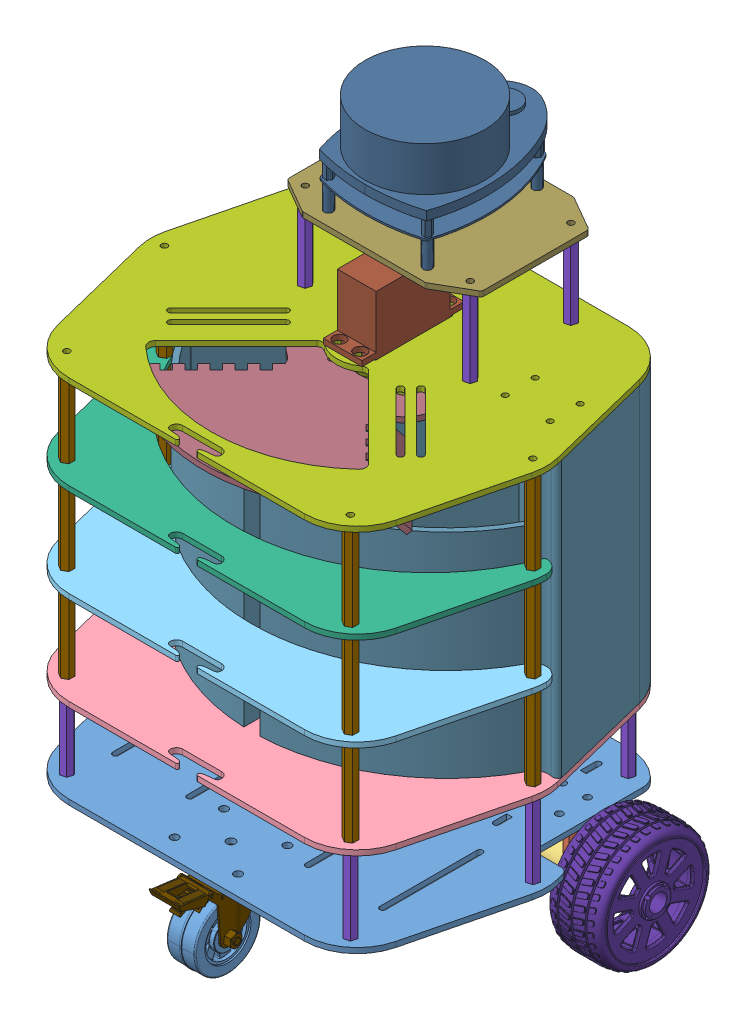
SolidWorks assembly 装配体1, configuration 默认. Lengths in mm.
Overall size (255.2 380.4 208.91).
45 component instances, 21 part files, 94 mates.
Components (placement in the parent):
- 底板1-1: 底板1 [默认] at origin size (224.29 3 183.94)
- 电机支架-1: 电机支架 [默认] at (90.25 -20.75 -110.5986) x (-1 0 0) z (0 0 1) size (33 34 26.5)
- 电机-1: 电机 [默认] at (36.95 -20.75 -110.5986) size (71 25.53 25.53)
- 电机-2: 电机 [默认] at (-36.95 -20.75 -110.5986) x (-1 0 0) z (0 0 -1) size (71 25.53 25.53)
- 电机支架-2: 电机支架 [默认] at (-90.25 -20.75 -110.5986) x (1 0 0) z (0 0 -1) size (33 34 26.5)
- 底板2-1: 底板2 [默认] at (0 48 0) size (224.29 3 183.94)
- 底板3-1: 底板3 [默认] at (0 101 0) size (224.29 3 99.61)
- 底板4-1: 底板4 [默认] at (0 154 0) size (224.29 3 99.54)
- 底板5-1: 底板5 [默认] at (0 207 0) size (224.29 3 183.94)
- 铜柱45-1: 铜柱45 [默认] at (80.4502 3 16.819) size (6.73 45 6.65)
- 铜柱45-2: 铜柱45 [默认] at (104.5075 3 -62.6242) size (6.73 45 6.65)
- 铜柱45-4: 铜柱45 [默认] at (-80.4502 3 16.819) size (6.73 45 6.65)
- 铜柱45-5: 铜柱45 [默认] at (-104.5075 3 -62.6242) size (6.73 45 6.65)
- 铜柱45-6: 铜柱45 [默认] at (-79.5 3 -141.7823) size (6.73 45 6.65)
- 铜柱45-7: 铜柱45 [默认] at (79.5 3 -141.7823) size (6.73 45 6.65)
- 铜柱50-1: 铜柱50 [默认] at (104.5075 157 -62.6242) size (6.07 50 6.93)
- 铜柱50-2: 铜柱50 [默认] at (-80.4502 51 16.819) size (6.07 50 6.93)
- 铜柱50-3: 铜柱50 [默认] at (-104.5075 51 -62.6242) size (6.07 50 6.93)
- 铜柱50-4: 铜柱50 [默认] at (80.4502 51 16.819) size (6.07 50 6.93)
- 铜柱50-5: 铜柱50 [默认] at (-104.5075 104 -62.6242) size (6.07 50 6.93)
- 铜柱50-6: 铜柱50 [默认] at (-80.4502 104 16.819) size (6.07 50 6.93)
- 铜柱50-7: 铜柱50 [默认] at (104.5075 51 -62.6242) size (6.07 50 6.93)
- 铜柱50-8: 铜柱50 [默认] at (80.4502 104 16.819) size (6.07 50 6.93)
- 铜柱50-9: 铜柱50 [默认] at (-80.4502 157 16.819) size (6.07 50 6.93)
- 铜柱50-10: 铜柱50 [默认] at (104.5075 104 -62.6242) size (6.07 50 6.93)
- 铜柱50-11: 铜柱50 [默认] at (-104.5075 157 -62.6242) size (6.07 50 6.93)
- 铜柱50-12: 铜柱50 [默认] at (80.4502 157 16.819) size (6.07 50 6.93)
- 激光雷达X4-1: 激光雷达X4 [默认] at (0 258 -120.1085) x (-1 0 0) z (0 0 -1) size (70.42 57 94.61)
- 舵机-1: 舵机 [默认] at (0 243 -88.1867) x (0 0 -1) z (-1 0 0) size (58 50 22)
- 底板6-1: 底板6 [默认] at (0.7291 255 -93.893) x (1 0 0) z (0 1 0) size (110.33 83.99 3)
- 铜柱45-8: 铜柱45 [默认] at (47.5277 210 -141.1486) size (6.73 45 6.65)
- 铜柱45-9: 铜柱45 [默认] at (-46.0695 210 -84.051) size (6.73 45 6.65)
- 铜柱45-10: 铜柱45 [默认] at (-46.0695 210 -141.1486) size (6.73 45 6.65)
- 铜柱45-11: 铜柱45 [默认] at (47.5277 210 -84.051) size (6.73 45 6.65)
- 乘物-1: 乘物 [默认] at (-0.1354 193 -20.9339) size (143.43 24.32 112.61)
- 垃圾桶-1: 垃圾桶 [默认] at (0.1354 51 -61.3346) size (220.93 156 146.93)
- 铜柱156-1: 铜柱156 [默认] at (0 51 -131.5682) size (6.91 156 6.21)
- 铜柱156-2: 铜柱156 [默认] at (0 51 -144.0797) size (6.91 156 6.21)
- 一字摇臂-1: 一字摇臂 [默认] at (0 193 -73.9628) x (1 0 0) z (0 1 0) size (47 9.8 7.5)
- 乘物2-1: 乘物2 [默认] at (47.7312 192.1451 -37.8905) x (0.651005 -0.382877 -0.655438) z (0.685403 -0.074582 0.724335) size (19.13 3 48.09) (hidden)
- 轮子酷-1: 轮子酷 [Default] at (-135.2789 -20.75 -110.5986) x (0 0.249093 0.96848) z (-1 0 0) size (66.95 66.95 31.63)
- 轮子酷-2: 轮子酷 [Default] at (135.2789 -20.75 -110.5986) x (0 0.432005 -0.901871) z (1 0 0) size (66.95 66.95 31.63)
- 万向-1: 万向 [默认] at (0 0 4.1514) x (0 0 -1) z (1 0 0) size (55.67 39.63 29.93)
- 万向新轮子-1: 万向新轮子 [默认] at (0.0227 -0.0918 24.1728) x (0 -0.009175 0.999958) z (-1 0 0) size (46.01 53.63 29.93)
- IMU-1: IMU [默认] at (-36.2463 19.5 -94.4147) size (55 18.5 65)
Mates (geometry in assembly coordinates):
- 同心1: concentric anti-aligned: cylinder of 电机支架-1 through (86.95 -20.75 -110.5986) axis (1 0 0) radius 4; cylinder of 电机-1 through (98.95 -20.75 -110.5986) axis (-1 0 0) radius 2
- 同心2: concentric aligned: cylinder of 电机支架-1 through (86.95 -20.75 -119.0986) axis (1 0 0) radius 1.5; cylinder of 电机-1 through (83.95 -20.75 -119.0986) axis (1 0 0) radius 1.5
- 重合1: coincident anti-aligned: plane of 电机支架-1 through (86.95 -20.75 -110.5986) normal (-1 0 0); plane of 电机-1 through (86.95 -20.75 -110.5986) normal (1 0 0)
- 重合3: coincident anti-aligned: plane of 底板1-1 through (0 0 0) normal (0 -1 0); plane of 电机支架-1 through (86.95 0 -97.3486) normal (0 1 0)
- 重合5: coincident anti-aligned: plane of 电机-2 through (-86.95 -20.75 -110.5986) normal (-1 0 0); plane of 电机支架-2 through (-86.95 -20.75 -110.5986) normal (1 0 0)
- 同心4: concentric anti-aligned: cylinder of 电机-2 through (-98.95 -20.75 -110.5986) axis (1 0 0) radius 2; cylinder of 电机支架-2 through (-86.95 -20.75 -110.5986) axis (-1 0 0) radius 4
- 同心6: concentric aligned: cylinder of 电机-2 through (-83.95 -20.75 -102.0986) axis (-1 0 0) radius 1.5; cylinder of 电机支架-2 through (-86.95 -20.75 -102.0986) axis (-1 0 0) radius 1.5
- 重合6: coincident aligned: plane of 底板1-1 through (90.25 3 0) normal (1 0 0); plane of 电机支架-1 through (90.25 -20.75 -110.5986) normal (1 0 0)
- 重合7: coincident anti-aligned: plane of 底板1-1 through (0 0 0) normal (0 -1 0); plane of 电机支架-2 through (-86.95 0 -123.8486) normal (0 1 0)
- 重合8: coincident aligned: plane of 底板1-1 through (-90.25 3 0) normal (-1 0 0); plane of 电机支架-2 through (-90.25 -20.75 -110.5986) normal (-1 0 0)
- 重合9: coincident aligned: plane of 电机支架-1 through (86.95 0 -123.8486) normal (0 0 -1); plane of 电机支架-2 through (-86.95 -20.75 -123.8486) normal (0 0 -1)
- 距离4: distance = 30.7453 mm aligned: plane of 电机支架-1 through (86.95 0 -123.8486) normal (0 0 -1); plane of 底板1-1 through (0 3 -154.594) normal (0 0 -1)
- 重合15: coincident aligned: plane of 底板1-1 through (91.8773 3 22.7831) normal (0.970604 0 0.240684); plane of 底板2-1 through (91.8773 51 22.7831) normal (0.970604 0 0.240684)
- 重合16: coincident aligned: plane of 底板1-1 through (0 3 29.3457) normal (0 0 1); plane of 底板2-1 through (0 51 29.3457) normal (0 0 1)
- 距离6: distance = 45 mm anti-aligned: plane of 底板1-1 through (0 3 0) normal (0 1 0); plane of 底板2-1 through (0 48 0) normal (0 -1 0)
- 重合18: coincident aligned: plane of 底板2-1 through (0 51 29.3457) normal (0 0 1); plane of 底板3-1 through (0 104 29.3457) normal (0 0 1)
- 重合19: coincident aligned: plane of 底板2-1 through (91.8773 51 22.7831) normal (0.970604 0 0.240684); plane of 底板3-1 through (91.8773 104 22.7831) normal (0.970604 0 0.240684)
- 重合20: coincident aligned: plane of 底板3-1 through (0 104 29.3457) normal (0 0 1); plane of 底板4-1 through (0 157 29.3457) normal (0 0 1)
- 重合21: coincident: plane of 底板3-1 through (91.8773 104 22.7831) normal (0.970604 0 0.240684); line of 底板4-1 through (95.8987 157 6.5662) axis (0.240684 0 -0.970604)
- 重合22: coincident aligned: plane of 底板4-1 through (91.8773 157 22.7831) normal (0.970604 0 0.240684); plane of 底板5-1 through (91.8773 210 22.7831) normal (0.970604 0 0.240684)
- 重合23: coincident aligned: plane of 底板4-1 through (0 157 29.3457) normal (0 0 1); plane of 底板5-1 through (0 210 29.3457) normal (0 0 1)
- 距离7: distance = 50 mm anti-aligned: plane of 底板2-1 through (0 51 0) normal (0 1 0); plane of 底板3-1 through (0 101 0) normal (0 -1 0)
- 距离8: distance = 50 mm anti-aligned: plane of 底板3-1 through (0 104 0) normal (0 1 0); plane of 底板4-1 through (0 154 0) normal (0 -1 0)
- 距离9: distance = 50 mm anti-aligned: plane of 底板5-1 through (0 207 0) normal (0 -1 0); plane of 底板4-1 through (0 157 0) normal (0 1 0)
- 同心8: concentric anti-aligned: cylinder of 底板2-1 through (104.5075 41 -62.6242) axis (0 1 0) radius 1.75; cylinder of 铜柱45-2 through (104.5075 48 -62.6242) axis (0 -1 0) radius 1.5
- 同心9: concentric anti-aligned: cylinder of 底板2-1 through (80.4502 41 16.819) axis (0 1 0) radius 1.75; cylinder of 铜柱45-1 through (80.4502 48 16.819) axis (0 -1 0) radius 1.5
- 同心10: concentric anti-aligned: cylinder of 底板2-1 through (-80.4502 41 16.819) axis (0 1 0) radius 1.75; cylinder of 铜柱45-4 through (-80.4502 48 16.819) axis (0 -1 0) radius 1.5
- 同心11: concentric anti-aligned: cylinder of 底板2-1 through (-104.5075 41 -62.6242) axis (0 1 0) radius 1.75; cylinder of 铜柱45-5 through (-104.5075 48 -62.6242) axis (0 -1 0) radius 1.5
- 重合28: coincident anti-aligned: plane of 底板1-1 through (0 3 0) normal (0 1 0); plane of 铜柱45-2 through (104.5075 3 -62.6242) normal (0 -1 0)
- 重合31: coincident anti-aligned: plane of 底板1-1 through (0 3 0) normal (0 1 0); plane of 铜柱45-1 through (80.4502 3 16.819) normal (0 -1 0)
- 重合32: coincident anti-aligned: plane of 底板1-1 through (0 3 0) normal (0 1 0); plane of 铜柱45-4 through (-80.4502 3 16.819) normal (0 -1 0)
- 重合33: coincident anti-aligned: plane of 底板1-1 through (0 3 0) normal (0 1 0); plane of 铜柱45-5 through (-104.5075 3 -62.6242) normal (0 -1 0)
- 同心14: concentric anti-aligned: cylinder of 底板3-1 through (104.5075 94 -62.6242) axis (0 1 0) radius 1.75; cylinder of 铜柱50-7 through (104.5075 101 -62.6242) axis (0 -1 0) radius 1.5
- 重合34: coincident anti-aligned: plane of 底板3-1 through (0 101 0) normal (0 -1 0); plane of 铜柱50-7 through (104.5075 101 -62.6242) normal (0 1 0)
- 同心15: concentric anti-aligned: cylinder of 底板3-1 through (80.4502 94 16.819) axis (0 1 0) radius 1.75; cylinder of 铜柱50-4 through (80.4502 101 16.819) axis (0 -1 0) radius 1.5
- 重合35: coincident anti-aligned: plane of 底板3-1 through (0 101 0) normal (0 -1 0); plane of 铜柱50-4 through (80.4502 101 16.819) normal (0 1 0)
- 同心16: concentric anti-aligned: cylinder of 底板3-1 through (-80.4502 94 16.819) axis (0 1 0) radius 1.75; cylinder of 铜柱50-2 through (-80.4502 101 16.819) axis (0 -1 0) radius 1.5
- 重合36: coincident anti-aligned: plane of 底板3-1 through (0 101 0) normal (0 -1 0); plane of 铜柱50-2 through (-80.4502 101 16.819) normal (0 1 0)
- 同心17: concentric anti-aligned: cylinder of 底板3-1 through (-104.5075 94 -62.6242) axis (0 1 0) radius 1.75; cylinder of 铜柱50-3 through (-104.5075 101 -62.6242) axis (0 -1 0) radius 1.5
- 重合37: coincident anti-aligned: plane of 底板3-1 through (0 101 0) normal (0 -1 0); plane of 铜柱50-3 through (-104.5075 101 -62.6242) normal (0 1 0)
- 重合38: coincident anti-aligned: plane of 底板4-1 through (0 154 0) normal (0 -1 0); plane of 铜柱50-5 through (-104.5075 154 -62.6242) normal (0 1 0)
- 同心18: concentric anti-aligned: cylinder of 底板4-1 through (-104.5075 147 -62.6242) axis (0 1 0) radius 1.75; cylinder of 铜柱50-5 through (-104.5075 154 -62.6242) axis (0 -1 0) radius 1.5
- 同心19: concentric anti-aligned: cylinder of 底板4-1 through (-80.4502 147 16.819) axis (0 1 0) radius 1.75; cylinder of 铜柱50-6 through (-80.4502 154 16.819) axis (0 -1 0) radius 1.5
- 重合40: coincident anti-aligned: plane of 底板4-1 through (0 154 0) normal (0 -1 0); plane of 铜柱50-6 through (-80.4502 154 16.819) normal (0 1 0)
- 重合41: coincident anti-aligned: plane of 底板4-1 through (0 154 0) normal (0 -1 0); plane of 铜柱50-8 through (80.4502 154 16.819) normal (0 1 0)
- 同心20: concentric anti-aligned: cylinder of 底板4-1 through (80.4502 147 16.819) axis (0 1 0) radius 1.75; cylinder of 铜柱50-8 through (80.4502 154 16.819) axis (0 -1 0) radius 1.5
- 同心21: concentric anti-aligned: cylinder of 底板4-1 through (104.5075 147 -62.6242) axis (0 1 0) radius 1.75; cylinder of 铜柱50-10 through (104.5075 154 -62.6242) axis (0 -1 0) radius 1.5
- 重合42: coincident anti-aligned: plane of 底板4-1 through (0 154 0) normal (0 -1 0); plane of 铜柱50-10 through (104.5075 154 -62.6242) normal (0 1 0)
- 同心22: concentric anti-aligned: cylinder of 底板5-1 through (104.5075 200 -62.6242) axis (0 1 0) radius 1.75; cylinder of 铜柱50-1 through (104.5075 207 -62.6242) axis (0 -1 0) radius 1.5
- 重合43: coincident anti-aligned: plane of 底板5-1 through (0 207 0) normal (0 -1 0); plane of 铜柱50-1 through (104.5075 207 -62.6242) normal (0 1 0)
- 同心23: concentric anti-aligned: cylinder of 底板5-1 through (80.4502 200 16.819) axis (0 1 0) radius 1.75; cylinder of 铜柱50-12 through (80.4502 207 16.819) axis (0 -1 0) radius 1.5
- 重合44: coincident anti-aligned: plane of 底板5-1 through (0 207 0) normal (0 -1 0); plane of 铜柱50-12 through (80.4502 207 16.819) normal (0 1 0)
- 同心24: concentric anti-aligned: cylinder of 底板5-1 through (-80.4502 200 16.819) axis (0 1 0) radius 1.75; cylinder of 铜柱50-9 through (-80.4502 207 16.819) axis (0 -1 0) radius 1.5
- 重合45: coincident anti-aligned: plane of 底板5-1 through (0 207 0) normal (0 -1 0); plane of 铜柱50-9 through (-80.4502 207 16.819) normal (0 1 0)
- 同心26: concentric anti-aligned: cylinder of 底板5-1 through (-104.5075 200 -62.6242) axis (0 1 0) radius 1.75; cylinder of 铜柱50-11 through (-104.5075 207 -62.6242) axis (0 -1 0) radius 1.5
- 重合46: coincident anti-aligned: plane of 底板5-1 through (0 207 0) normal (0 -1 0); plane of 铜柱50-11 through (-104.5075 207 -62.6242) normal (0 1 0)
- 重合48: coincident anti-aligned: plane of 激光雷达X4-1 through (0 258 -120.1085) normal (-1 0 0); plane of assembly through (0 0 0) normal (1 0 0)
- 同心27: concentric aligned: cylinder of 底板5-1 through (0 200 -73.9628) axis (0 1 0) radius 18; cylinder of 舵机-1 through (0 193 -73.9628) axis (0 1 0) radius 4.5817
- 重合52: coincident anti-aligned: plane of 底板5-1 through (0 210 0) normal (0 1 0); plane of 舵机-1 through (0 210 -88.1867) normal (0 -1 0)
- 平行3: parallel anti-aligned: plane of 底板5-1 through (0 210 0) normal (0 1 0); plane of 底板6-1 through (-52.4384 255 -83.404) normal (0 -1 0)
- 重合56: coincident aligned: plane of 底板5-1 through (0 210 -154.594) normal (0 0 -1); plane of 底板6-1 through (35.1932 141.2861 -154.594) normal (0 0 -1)
- 距离10: distance = 45 mm anti-aligned: plane of 底板6-1 through (-52.4384 255 -83.404) normal (0 -1 0); plane of 底板5-1 through (0 210 0) normal (0 1 0)
- 重合58: coincident anti-aligned: plane of 激光雷达X4-1 through (-19.6955 258 -149.0549) normal (0 -1 0); plane of 底板6-1 through (-52.4384 258 -83.404) normal (0 1 0)
- 同心28: concentric anti-aligned: cylinder of 底板2-1 through (-79.5 41 -141.7823) axis (0 1 0) radius 1.75; cylinder of 铜柱45-6 through (-79.5 48 -141.7823) axis (0 -1 0) radius 1.5
- 同心29: concentric anti-aligned: cylinder of 底板2-1 through (79.5 41 -141.7823) axis (0 1 0) radius 1.75; cylinder of 铜柱45-7 through (79.5 48 -141.7823) axis (0 -1 0) radius 1.5
- 同心30: concentric anti-aligned: circle of 底板5-1; cylinder of 铜柱45-9 through (-46.0695 255 -84.051) axis (0 -1 0) radius 1.5
- 同心31: concentric anti-aligned: cylinder of 底板6-1 through (47.5277 248 -141.1486) axis (0 1 0) radius 1.75; cylinder of 铜柱45-8 through (47.5277 255 -141.1486) axis (0 -1 0) radius 1.5
- 重合59: coincident anti-aligned: plane of 底板6-1 through (-52.4384 255 -83.404) normal (0 -1 0); plane of 铜柱45-8 through (47.5277 255 -141.1486) normal (0 1 0)
- 重合60: coincident anti-aligned: plane of 底板6-1 through (-52.4384 255 -83.404) normal (0 -1 0); plane of 铜柱45-9 through (-46.0695 255 -84.051) normal (0 1 0)
- 同心32: concentric anti-aligned: cylinder of 底板6-1 through (-46.0695 248 -141.1486) axis (0 1 0) radius 1.75; cylinder of 铜柱45-10 through (-46.0695 255 -141.1486) axis (0 -1 0) radius 1.5
- 重合61: coincident anti-aligned: plane of 底板6-1 through (-52.4384 255 -83.404) normal (0 -1 0); plane of 铜柱45-10 through (-46.0695 255 -141.1486) normal (0 1 0)
- 同心33: concentric anti-aligned: cylinder of 底板6-1 through (47.5277 248 -84.051) axis (0 1 0) radius 1.75; cylinder of 铜柱45-11 through (47.5277 255 -84.051) axis (0 -1 0) radius 1.5
- 重合62: coincident anti-aligned: plane of 底板6-1 through (-52.4384 255 -83.404) normal (0 -1 0); plane of 铜柱45-11 through (47.5277 255 -84.051) normal (0 1 0)
- 重合63: coincident aligned: plane of 舵机-1 through (0 193 -73.9628) normal (0 -1 0); plane of 乘物-1 through (-0.1354 193 -20.9339) normal (0 -1 0)
- 同心34: concentric anti-aligned: cylinder of 底板5-1 through (0 200 -131.5682) axis (0 1 0) radius 1.75; cylinder of 铜柱156-1 through (0 207 -131.5682) axis (0 -1 0) radius 1.5
- 重合64: coincident anti-aligned: plane of 底板5-1 through (0 207 0) normal (0 -1 0); plane of 铜柱156-1 through (0 207 -131.5682) normal (0 1 0)
- 同心35: concentric anti-aligned: cylinder of 底板5-1 through (0 200 -144.0797) axis (0 1 0) radius 1.75; cylinder of 铜柱156-2 through (0 207 -144.0797) axis (0 -1 0) radius 1.5
- 重合65: coincident anti-aligned: plane of 底板5-1 through (0 207 0) normal (0 -1 0); plane of 铜柱156-2 through (0 207 -144.0797) normal (0 1 0)
- 重合66: coincident anti-aligned: plane of 底板2-1 through (0 51 0) normal (0 1 0); plane of 垃圾桶-1 through (0.1354 51 -61.3346) normal (0 -1 0)
- 同心36: concentric anti-aligned: cylinder of 舵机-1 through (0 193 -73.9628) axis (0 1 0) radius 4.5817; cylinder of 一字摇臂-1 through (0 195.5 -73.9628) axis (0 -1 0) radius 3
- 平行4: parallel anti-aligned: plane of 一字摇臂-1 through (0 193 -73.9628) normal (0 0 -1); plane of assembly through (0 0 0) normal (0 0 1)
- 重合69: coincident aligned: plane of 乘物-1 through (-0.1354 193 -20.9339) normal (0 -1 0); plane of 一字摇臂-1 through (0 193 -73.9628) normal (0 -1 0)
- 同心38: concentric aligned: cylinder of 电机-2 through (-98.95 -20.75 -110.5986) axis (1 0 0) radius 2; cone of 轮子酷-1 through (-120.25 -20.75 -110.5986) axis (1 0 0)
- 同心39: concentric aligned: cylinder of 电机-1 through (98.95 -20.75 -110.5986) axis (-1 0 0) radius 2; cone of 轮子酷-2 through (120.25 -20.75 -110.5986) axis (-1 0 0)
- 距离11: distance = 6 mm anti-aligned: plane of 底板1-1 through (90.25 3 0) normal (1 0 0); plane of 轮子酷-2 through (96.25 -20.75 -110.5986) normal (-1 0 0)
- 距离12: distance = 6 mm anti-aligned: plane of 轮子酷-1 through (-96.25 -20.75 -110.5986) normal (1 0 0); plane of 底板1-1 through (-90.25 3 0) normal (-1 0 0)
- 同心40: concentric anti-aligned: cylinder of 底板1-1 through (0 3 4.1514) axis (0 -1 0) radius 2.4148; cylinder of 万向-1 through (0 -3.7897 4.1514) axis (0 1 0) radius 3.4486
- 重合72: coincident anti-aligned: plane of 底板1-1 through (0 0 0) normal (0 -1 0); plane of 万向-1 through (-14.9655 0 21.349) normal (0 1 0)
- 平行6: parallel aligned: plane of 底板1-1 through (0 3 29.3457) normal (0 0 1); plane of 万向-1 through (12.1232 0 21.3489) normal (0 0 1)
- 同心41: concentric anti-aligned: cylinder of 万向-1 through (-9.0043 -34.6377 14.0034) axis (1 0 0) radius 1.8948; cylinder of 万向新轮子-1 through (8.1099 -34.6377 14.0034) axis (-1 0 0) radius 2.3685
- 宽度2: width anti-aligned: plane of 万向新轮子-1 through (-8.1099 -42.1213 13.5442) normal (-1 0 0); plane of 万向新轮子-1 through (8.1099 -42.1213 13.5442) normal (1 0 0); plane of 万向-1 through (-8.1327 -7.5034 25.9677) normal (1 0 0); plane of 万向-1 through (8.1327 -7.4404 9.0114) normal (-1 0 0)
- 重合73: coincident anti-aligned: plane of 底板1-1 through (0 3 0) normal (0 1 0); plane of IMU-1 through (-36.2463 3 -94.4147) normal (0 -1 0)
- 重合74: coincident aligned: plane of 底板1-1 through (-20.6886 -7 -67.1866) normal (0 0 1); plane of IMU-1 through (-62.1283 3 -67.1866) normal (0 0 1)
- 距离13: distance = 12 mm aligned: plane of IMU-1 through (-62.1283 3 -67.1866) normal (-1 0 0); plane of 底板1-1 through (-74.1283 -7 -61.2346) normal (-1 0 0)
